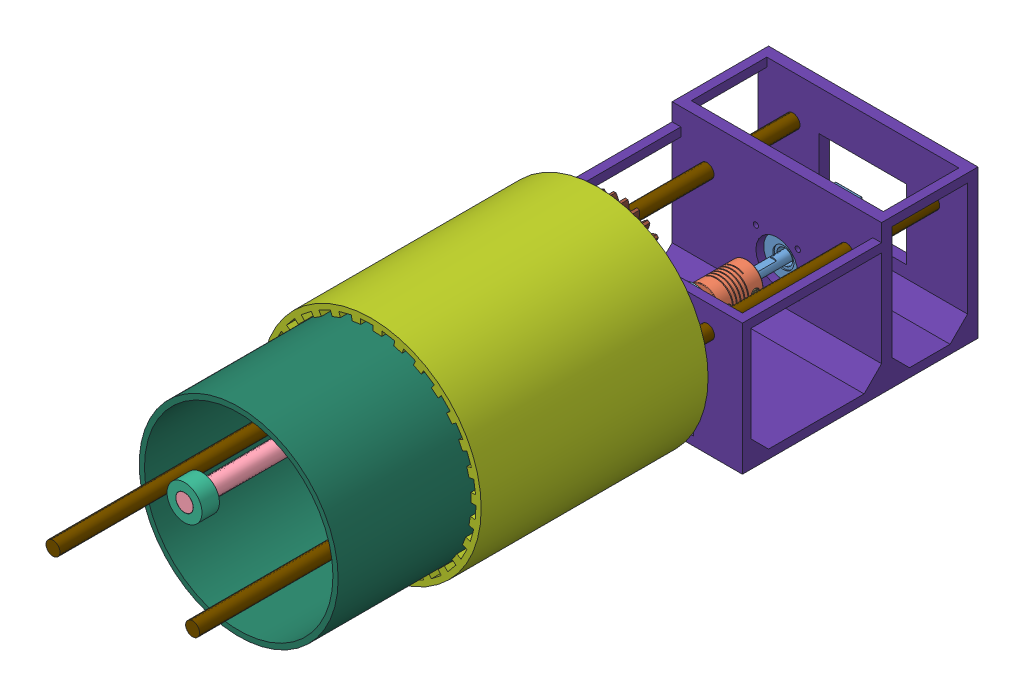
SolidWorks assembly Telescopic arm v2, configuration Default. Lengths in mm.
Overall size (126 126 430).
38 component instances, 19 part files, 60 mates.
Components (placement in the parent):
- NEMA 17-1: NEMA 17 [Default] at (17.8958 42.2414 18.8827) size (30 34.5 66.16)
- Flexible Coupler 5 to 10mm Assembly-2: Flexible Coupler 5 to 10mm Assembly [Default] at (21.8958 38.2414 89.3327) x (1 0 0) z (0 -1 0) size (20.23 25 20.36)
  - Flexible Coupler Body-1-1: Flexible Coupler Body-1 [Default] at origin size (19.87 25 19.54)
  - Set Screw M4x6mm-1-1: Set Screw M4x6mm-1 [Default] at (4 8 0) x (0 0.343805 0.939041) z (0 0.939041 -0.343805) size (4.09 6.29 4.71)
  - Set Screw M4x6mm-1-2: Set Screw M4x6mm-1 [Default] at (0 8 4.2969) x (0.669207 -0.743076 0) z (-0.743076 -0.669207 0) size (4.09 6.29 4.71)
  - Set Screw M4x6mm-1-3: Set Screw M4x6mm-1 [Default] at (0 -8 3.6) x (0.696812 -0.717254 0) z (-0.717254 -0.696812 0) size (4.09 6.29 4.71)
  - Set Screw M4x6mm-1-4: Set Screw M4x6mm-1 [Default] at (3.9139 -8 0) x (0 0.90109 0.433632) z (0 0.433632 -0.90109) size (4.09 6.29 4.71)
- T10 Lead Screw-1: T10 Lead Screw [Default] at (21.8958 38.2414 84.3327) x (-0.072732 0.997352 0) z (0.997352 0.072732 0) size (9.9 185 9.9)
- Endstop setter-1: Endstop setter [Default] at (21.8958 13.2414 121.8327) x (-1 0 0) z (0 0 1) size (60 43.3 30)
- Endstop-1: Endstop [Default] at (21.8958 38.2414 117.8327) x (1 0 0) z (0 1 0) size (20 10 20)
- Endstop-2: Endstop [Default] at (21.8958 38.2414 146.8327) x (1 0 0) z (0 1 0) size (20 10 20)
- Endstop-3: Endstop [Default] at (21.8958 38.2414 269.3327) x (1 0 0) z (0 1 0) size (20 10 20)
- Copy of Outer Shell Circular^Telescopic arm v2-1: Copy of Outer Shell Circular^Telescopic arm v2 [Default] at (21.8958 63.2414 161.9685) x (0 -1 0) z (0 0 -1) size (126 126 130) (virtual)
- T10 Lead nut-1: T10 Lead nut [Default] at (21.8958 38.2414 181.9685) x (0.838588 0.544766 0) z (0.544766 -0.838588 0) size (32 19 32)
- LeadNut coupler-1: LeadNut coupler [Default] at (0.9311 24.6222 181.9685) x (0.838588 0.544766 0) z (0 0 1) size (35 35 25)
- Spur Gear A^TelescopicArm-1: Spur Gear A^TelescopicArm [Default] at (0.591 25.0128 148.9685) x (0.838588 0.544766 0) z (0 0 1) size (54.73 54.83 8.1)
- Spur Gear B^TelescopicArm-1: Spur Gear B^TelescopicArm [Default] at (-3.1127 90.1018 148.9685) x (0.998553 -0.053779 0) z (0 0 1) size (54.73 54.83 8.1)
- Copy of Shaft B Gear^Telescopic arm v2-1: Copy of Shaft B Gear^Telescopic arm v2 [Default] at (21.8958 88.2414 183.9685) x (0.260682 -0.965425 0) z (0 0 1) size (12 12 72) (virtual)
- SKF_608-2ZZ.step-1: SKF_608-2ZZ.step [Default] at (21.8958 88.2414 183.9685) x (0 0 -1) z (0 1 0) size (7 22 22)
- Copy of Bearing Cap^Telescopic arm v2-1: Copy of Bearing Cap^Telescopic arm v2 [Default] at (46.8958 88.2414 186.9685) x (-1 0 0) z (0 0 1) size (36 36 7.9) (virtual)
- Flexible Coupler 5 to 10mm Assembly-3: Flexible Coupler 5 to 10mm Assembly [Default] at (21.8958 88.2414 218.9685) x (0.260682 -0.965425 0) z (-0.965425 -0.260682 0) size (20.23 25 20.36)
  - Flexible Coupler Body-1-1: Flexible Coupler Body-1 [Default] at origin size (19.87 25 19.54)
  - Set Screw M4x6mm-1-1: Set Screw M4x6mm-1 [Default] at (4 8 0) x (0 0.343805 0.939041) z (0 0.939041 -0.343805) size (4.09 6.29 4.71)
  - Set Screw M4x6mm-1-2: Set Screw M4x6mm-1 [Default] at (0 8 4.2969) x (0.669207 -0.743076 0) z (-0.743076 -0.669207 0) size (4.09 6.29 4.71)
  - Set Screw M4x6mm-1-3: Set Screw M4x6mm-1 [Default] at (0 -8 3.6) x (0.696812 -0.717254 0) z (-0.717254 -0.696812 0) size (4.09 6.29 4.71)
  - Set Screw M4x6mm-1-4: Set Screw M4x6mm-1 [Default] at (3.9139 -8 0) x (0 0.90109 0.433632) z (0 0.433632 -0.90109) size (4.09 6.29 4.71)
- T10 Lead Screw-2: T10 Lead Screw [Default] at (21.8958 88.2414 213.9685) x (0.770216 -0.637784 0) z (-0.637784 -0.770216 0) size (9.9 185 9.9)
- Endstop-4: Endstop [Default] at (21.8958 88.2414 398.9685) x (0.811964 -0.583707 0) z (0.583707 0.811964 0) size (20 10 20)
- T10 Lead nut-2: T10 Lead nut [Default] at (21.8958 88.2414 257.9254) x (1 0 0) z (0 -1 0) size (32 19 32)
- Inner Shell Circular-1: Inner Shell Circular [Default] at (21.8958 88.2414 237.9254) x (1 0 0) z (0 0 -1) size (114 114 130)
- RJMP_01_08_1-1: RJMP_01_08_1 [Default] at (61.8958 63.2414 168.9685) x (0.997604 -0.069187 0) z (-0.069187 -0.997604 0) size (16.01 25.01 16.01)
- RJMP_01_08_1-2: RJMP_01_08_1 [Default] at (-18.1042 63.2414 173.8535) x (1 0 0) z (0 -1 0) size (16.01 25.01 16.01)
- RJMP_01_08_1-3: RJMP_01_08_1 [Default] at (-18.1042 63.2414 244.9254) x (-0.177241 -0.984167 0) z (-0.984167 0.177241 0) size (16.01 25.01 16.01)
- RJMP_01_08_1-4: RJMP_01_08_1 [Default] at (61.8958 63.2414 244.9254) x (0.353226 -0.935538 0) z (-0.935538 -0.353226 0) size (16.01 25.01 16.01)
- Motor Mount^Telescopic arm v2-1: Motor Mount^Telescopic arm v2 [Default] at (21.8958 7.4414 121.8327) x (-1 0 0) z (0 0 1) size (120 85 135) (virtual)
- Guides 8mm-1: Guides 8mm [Default] at (61.8958 63.2414 4.3327) x (0.992169 -0.124902 0) z (0 0 1) size (8 8 430)
- Guides 8mm-2: Guides 8mm [Default] at (-18.1042 63.2414 4.3327) x (-0.277145 -0.960828 0) z (0 0 1) size (8 8 430)
- RJ4JP_01_08_1-1: RJ4JP_01_08_1 [Default] at (-18.1042 63.2414 169.6185) x (-0.179236 0.983806 0) z (0.983806 0.179236 0) size (15.01 24.01 15.01)
Mates (geometry in assembly coordinates):
- Concentric2: concentric anti-aligned: cylinder of NEMA 17-1 through (21.8958 38.2414 55.8327) axis (0 0 1) radius 3; cylinder of Flexible Coupler 5 to 10mm Assembly-2/Flexible Coupler Body-1-1 through (21.8958 38.2414 101.8327) axis (0 0 -1) radius 9.5
- Distance3: distance = 0 mm aligned: plane of Flexible Coupler 5 to 10mm Assembly-2/Flexible Coupler Body-1-1 through (21.8958 38.2414 84.3327) normal (0 0 1); plane of NEMA 17-1 through (21.8958 38.2414 84.3327) normal (0 0 1)
- Concentric3: concentric anti-aligned: cylinder of Flexible Coupler 5 to 10mm Assembly-2/Flexible Coupler Body-1-1 through (21.8958 38.2414 84.3327) axis (0 0 1) radius 5; cylinder of T10 Lead Screw-1 through (21.8958 38.2414 269.3327) axis (0 0 -1) radius 4.95
- Coincident4: coincident anti-aligned: plane of Flexible Coupler 5 to 10mm Assembly-2/Flexible Coupler Body-1-1 through (21.8958 38.2414 84.3327) normal (0 0 1); plane of T10 Lead Screw-1 through (21.8958 38.2414 84.3327) normal (0 0 -1)
- Concentric4: concentric aligned: cylinder of T10 Lead Screw-1 through (21.8958 38.2414 269.3327) axis (0 0 -1) radius 4.95; cylinder of Endstop setter-1 through (21.8958 38.2414 136.8327) axis (0 0 -1) radius 5.1
- Distance4: distance = 5 mm anti-aligned: plane of Endstop setter-1 through (51.8958 7.4414 106.8327) normal (0 0 -1); plane of Flexible Coupler 5 to 10mm Assembly-2/Flexible Coupler Body-1-1 through (21.8958 38.2414 101.8327) normal (0 0 1)
- Concentric5: concentric anti-aligned: cylinder of Endstop setter-1 through (21.8958 38.2414 117.8327) axis (0 0 -1) radius 10.75; cylinder of Endstop-1 through (21.8958 38.2414 107.8327) axis (0 0 1) radius 5.025
- Coincident6: coincident anti-aligned: plane of Endstop setter-1 through (21.8958 38.2414 117.8327) normal (0 0 -1); plane of Endstop-1 through (21.8958 38.2414 117.8327) normal (0 0 1)
- Concentric6: concentric anti-aligned: cylinder of Endstop setter-1 through (21.8958 38.2414 136.8327) axis (0 0 -1) radius 10; cylinder of Endstop-2 through (21.8958 38.2414 136.8327) axis (0 0 1) radius 5.025
- Coincident7: coincident anti-aligned: plane of Endstop setter-1 through (51.8958 7.4414 136.8327) normal (0 0 1); plane of Endstop-2 through (21.8958 38.2414 136.8327) normal (0 0 -1)
- Concentric8: concentric anti-aligned: cylinder of T10 Lead Screw-1 through (21.8958 38.2414 269.3327) axis (0 0 -1) radius 4.95; cylinder of Endstop-3 through (21.8958 38.2414 259.3327) axis (0 0 1) radius 5.025
- Coincident8: coincident aligned: plane of T10 Lead Screw-1 through (21.8958 38.2414 269.3327) normal (0 0 1); plane of Endstop-3 through (21.8958 38.2414 269.3327) normal (0 0 1)
- Concentric12: concentric aligned: cylinder of T10 Lead Screw-1 through (21.8958 38.2414 269.3327) axis (0 0 -1) radius 4.95; cylinder of T10 Lead nut-1 through (21.8958 38.2414 200.9695) axis (0 0 -1) radius 5
- Concentric13: concentric anti-aligned: cylinder of T10 Lead nut-1 through (21.8958 38.2414 200.9695) axis (0 0 -1) radius 5; cylinder of LeadNut coupler-1 through (21.8958 38.2414 156.9685) axis (0 0 1) radius 5.5
- Concentric14: concentric anti-aligned: cylinder of T10 Lead nut-1 through (11.8327 31.7042 200.9695) axis (0 0 -1) radius 1.9; cylinder of LeadNut coupler-1 through (11.8327 31.7042 156.9675) axis (0 0 1) radius 2.1
- Coincident10: coincident anti-aligned: plane of T10 Lead nut-1 through (21.8958 38.2414 181.9685) normal (0 0 -1); plane of LeadNut coupler-1 through (0.9311 24.6222 181.9685) normal (0 0 1)
- Coincident11: coincident anti-aligned: plane of Copy of Outer Shell Circular^Telescopic arm v2-1 through (21.8958 38.2414 181.9685) normal (0 0 -1); plane of LeadNut coupler-1 through (0.9311 24.6222 181.9685) normal (0 0 1)
- Concentric15: concentric anti-aligned: cylinder of Copy of Outer Shell Circular^Telescopic arm v2-1 through (21.8958 38.2414 181.9685) axis (0 0 -1) radius 21; cylinder of LeadNut coupler-1 through (21.8958 38.2414 156.9685) axis (0 0 1) radius 5.5
- Concentric16: concentric aligned: cylinder of LeadNut coupler-1 through (21.8958 38.2414 -118.0315) axis (0 0 1) radius 17.5; cylinder of Spur Gear A^TelescopicArm-1 through (21.8958 38.2414 146.9685) axis (0 0 1) radius 5.5
- Concentric17: concentric aligned: cylinder of LeadNut coupler-1 through (28.4329 28.1783 156.9675) axis (0 0 1) radius 2.1; cylinder of Spur Gear A^TelescopicArm-1 through (28.4329 28.1783 148.8685) axis (0 0 1) radius 2
- Coincident12: coincident anti-aligned: plane of LeadNut coupler-1 through (0.9311 24.6222 156.9685) normal (0 0 -1); plane of Spur Gear A^TelescopicArm-1 through (21.8957 38.2414 156.9685) normal (0 0 1)
- Concentric18: concentric aligned: cylinder of Copy of Outer Shell Circular^Telescopic arm v2-1 through (21.8958 88.2414 186.9685) axis (0 0 -1) radius 9; cylinder of Spur Gear B^TelescopicArm-1 through (21.8958 88.2414 156.9695) axis (0 0 -1) radius 3
- Concentric19: concentric anti-aligned: cylinder of Spur Gear B^TelescopicArm-1 through (21.8958 88.2414 156.9695) axis (0 0 -1) radius 3; cylinder of Copy of Shaft B Gear^Telescopic arm v2-1 through (21.8958 88.2414 141.9685) axis (0 0 1) radius 3
- Coincident15: coincident anti-aligned: plane of Spur Gear B^TelescopicArm-1 through (21.8957 88.2414 156.9685) normal (0 0 1); plane of Copy of Shaft B Gear^Telescopic arm v2-1 through (21.8958 88.2414 156.9685) normal (0 0 -1)
- Concentric20: concentric aligned: cylinder of Copy of Outer Shell Circular^Telescopic arm v2-1 through (21.8958 88.2414 176.9685) axis (0 0 1) radius 11.04; cylinder of SKF_608-2ZZ.step-1 through (21.8958 88.2414 133.9685) axis (0 0 1) radius 11
- Coincident16: coincident anti-aligned: plane of Copy of Outer Shell Circular^Telescopic arm v2-1 through (21.8958 88.2414 176.9685) normal (0 0 1); plane of SKF_608-2ZZ.step-1 through (12.2958 88.2414 176.9685) normal (0 0 -1)
- Coincident17: coincident anti-aligned: plane of Copy of Shaft B Gear^Telescopic arm v2-1 through (21.8958 88.2414 183.9685) normal (0 0 -1); plane of SKF_608-2ZZ.step-1 through (15.9208 88.2414 183.9685) normal (0 0 1)
- Concentric21: concentric anti-aligned: cylinder of Copy of Outer Shell Circular^Telescopic arm v2-1 through (21.8958 88.2414 176.9685) axis (0 0 1) radius 11.04; cylinder of Copy of Bearing Cap^Telescopic arm v2-1 through (21.8958 88.2414 191.9685) axis (0 0 -1) radius 18
- Concentric22: concentric anti-aligned: cylinder of Copy of Outer Shell Circular^Telescopic arm v2-1 through (7.8958 88.2414 291.9695) axis (0 0 -1) radius 1.5; cylinder of Copy of Bearing Cap^Telescopic arm v2-1 through (7.8958 88.2414 184.0675) axis (0 0 1) radius 1.5
- Coincident18: coincident anti-aligned: plane of Copy of Outer Shell Circular^Telescopic arm v2-1 through (21.8958 63.2414 186.9685) normal (0 0 1); plane of Copy of Bearing Cap^Telescopic arm v2-1 through (21.8958 88.2414 186.9685) normal (0 0 -1)
- Concentric23: concentric anti-aligned: cylinder of Copy of Shaft B Gear^Telescopic arm v2-1 through (21.8958 88.2414 156.9685) axis (0 0 1) radius 4.1; cylinder of Flexible Coupler 5 to 10mm Assembly-3/Flexible Coupler Body-1-1 through (21.8958 88.2414 231.4685) axis (0 0 -1) radius 9.5
- Coincident20: coincident aligned: plane of Copy of Shaft B Gear^Telescopic arm v2-1 through (21.8958 88.2414 213.9685) normal (0 0 1); plane of Flexible Coupler 5 to 10mm Assembly-3/Flexible Coupler Body-1-1 through (21.8958 88.2414 213.9685) normal (0 0 1)
- Concentric24: concentric anti-aligned: cylinder of Flexible Coupler 5 to 10mm Assembly-3/Flexible Coupler Body-1-1 through (21.8958 88.2414 213.9685) axis (0 0 1) radius 5; cylinder of T10 Lead Screw-2 through (21.8958 88.2414 398.9685) axis (0 0 -1) radius 4.95
- Coincident21: coincident anti-aligned: plane of Flexible Coupler 5 to 10mm Assembly-3/Flexible Coupler Body-1-1 through (21.8958 88.2414 213.9685) normal (0 0 1); plane of T10 Lead Screw-2 through (21.8958 88.2414 213.9685) normal (0 0 -1)
- Concentric28: concentric anti-aligned: cylinder of T10 Lead Screw-2 through (21.8958 88.2414 398.9685) axis (0 0 -1) radius 4.95; cylinder of Endstop-4 through (21.8958 88.2414 388.9685) axis (0 0 1) radius 10
- Coincident22: coincident aligned: plane of T10 Lead Screw-2 through (21.8958 88.2414 398.9685) normal (0 0 1); plane of Endstop-4 through (21.8958 88.2414 398.9685) normal (0 0 1)
- Concentric30: concentric aligned: cylinder of T10 Lead Screw-2 through (21.8958 88.2414 398.9685) axis (0 0 -1) radius 4.95; cylinder of T10 Lead nut-2 through (21.8958 88.2414 276.9254) axis (0 0 -1) radius 8
- Concentric31: concentric aligned: cylinder of T10 Lead nut-2 through (21.8958 88.2414 276.9254) axis (0 0 -1) radius 8; cylinder of Inner Shell Circular-1 through (21.8958 88.2414 257.9254) axis (0 0 -1) radius 5.25
- Concentric32: concentric aligned: cylinder of T10 Lead nut-2 through (33.8958 88.2414 276.9264) axis (0 0 -1) radius 1.9; cylinder of Inner Shell Circular-1 through (33.8958 88.2414 257.9254) axis (0 0 -1) radius 2
- Coincident23: coincident anti-aligned: plane of T10 Lead nut-2 through (21.8958 88.2414 257.9254) normal (0 0 -1); plane of Inner Shell Circular-1 through (21.8958 63.2414 257.9254) normal (0 0 1)
- Coincident24: coincident aligned: plane of RJMP_01_08_1-1 through (70.4301 70.6687 175.9685) normal (0 0 1); plane of Copy of Outer Shell Circular^Telescopic arm v2-1 through (61.8958 63.2414 175.9685) normal (0 0 1)
- Concentric33: concentric aligned: cylinder of Copy of Outer Shell Circular^Telescopic arm v2-1 through (61.8958 63.2414 181.4685) axis (0 0 -1) radius 8; line of RJMP_01_08_1-1 through (61.8958 63.2414 181.4685) axis (0 0 -1)
- Concentric35: concentric aligned: cylinder of Inner Shell Circular-1 through (-18.1042 63.2414 257.4254) axis (0 0 -1) radius 8; line of RJMP_01_08_1-3 through (-18.1042 63.2414 257.4254) axis (0 0 -1)
- Concentric36: concentric aligned: cylinder of Inner Shell Circular-1 through (61.8958 63.2414 257.4254) axis (0 0 -1) radius 8; line of RJMP_01_08_1-4 through (61.8958 63.2414 257.4254) axis (0 0 -1)
- Concentric41: concentric aligned: cylinder of Copy of Outer Shell Circular^Telescopic arm v2-1 through (61.8958 63.2414 181.4685) axis (0 0 -1) radius 8; cylinder of Inner Shell Circular-1 through (61.8958 63.2414 257.4254) axis (0 0 -1) radius 8
- Concentric46: concentric aligned: cylinder of Endstop setter-1 through (1.8958 7.2414 121.8327) axis (0 1 0) radius 2.6; cylinder of Motor Mount^Telescopic arm v2-1 through (1.8958 2.4404 121.8327) axis (0 1 0) radius 2.6
- Concentric47: concentric aligned: cylinder of Endstop setter-1 through (41.8958 7.2414 121.8327) axis (0 1 0) radius 2.6; cylinder of Motor Mount^Telescopic arm v2-1 through (41.8958 2.4404 121.8327) axis (0 1 0) radius 2.6
- Coincident29: coincident anti-aligned: plane of Endstop setter-1 through (21.8958 7.4414 121.8327) normal (0 -1 0); plane of Motor Mount^Telescopic arm v2-1 through (21.8958 7.4414 121.8327) normal (0 1 0)
- Concentric48: concentric aligned: cylinder of Motor Mount^Telescopic arm v2-1 through (61.8958 63.2414 139.3327) axis (0 0 -1) radius 4; cylinder of Guides 8mm-1 through (61.8958 63.2414 434.3327) axis (0 0 -1) radius 4
- Coincident31: coincident aligned: plane of Motor Mount^Telescopic arm v2-1 through (81.8958 7.4414 4.3327) normal (0 0 -1); plane of Guides 8mm-1 through (61.8958 63.2414 4.3327) normal (0 0 -1)
- Concentric49: concentric aligned: cylinder of Motor Mount^Telescopic arm v2-1 through (-18.1042 63.2414 139.3327) axis (0 0 -1) radius 4; cylinder of Guides 8mm-2 through (-18.1042 63.2414 434.3327) axis (0 0 -1) radius 4
- Coincident32: coincident aligned: plane of Motor Mount^Telescopic arm v2-1 through (81.8958 7.4414 4.3327) normal (0 0 -1); plane of Guides 8mm-2 through (-18.1042 63.2414 4.3327) normal (0 0 -1)
- Parallel6: parallel aligned: cylinder of Copy of Outer Shell Circular^Telescopic arm v2-1 through (61.8958 63.2414 181.4685) axis (0 0 -1) radius 8; cylinder of Guides 8mm-1 through (61.8958 63.2414 434.3327) axis (0 0 -1) radius 4
- Concentric51: concentric aligned: cylinder of Copy of Outer Shell Circular^Telescopic arm v2-1 through (61.8958 63.2414 181.4685) axis (0 0 -1) radius 8; cylinder of Guides 8mm-1 through (61.8958 63.2414 434.3327) axis (0 0 -1) radius 4
- Concentric52: concentric anti-aligned: cylinder of Guides 8mm-2 through (-18.1042 63.2414 434.3327) axis (0 0 -1) radius 4; cylinder of Copy of Outer Shell Circular^Telescopic arm v2-1 through (-18.1042 63.2414 175.9685) axis (0 0 1) radius 13
- Parallel7: parallel aligned: plane of NEMA 17-1 through (21.8958 18.7414 25.6827) normal (0 -1 0); plane of Motor Mount^Telescopic arm v2-1 through (21.8958 2.4414 121.8327) normal (0 -1 0)
- Concentric53: concentric aligned: cylinder of Copy of Outer Shell Circular^Telescopic arm v2-1 through (-18.1042 63.2414 181.4685) axis (0 0 -1) radius 7.5; line of RJ4JP_01_08_1-1 through (-18.1042 63.2414 181.6185) axis (0 0 -1)
- Coincident33: coincident aligned: plane of Copy of Outer Shell Circular^Telescopic arm v2-1 through (21.8958 63.2414 161.9685) normal (0 0 -1); plane of RJ4JP_01_08_1-1 through (-24.1385 54.5186 161.9685) normal (0 0 -1)
- Coincident34: coincident aligned: plane of Inner Shell Circular-1 through (21.8958 63.2414 237.9254) normal (0 0 -1); plane of RJMP_01_08_1-4 through (66.5542 73.5515 237.9254) normal (0 0 -1)
- Coincident35: coincident aligned: plane of Inner Shell Circular-1 through (21.8958 63.2414 237.9254) normal (0 0 -1); plane of RJMP_01_08_1-3 through (-8.813 69.6968 237.9254) normal (0 0 -1)
